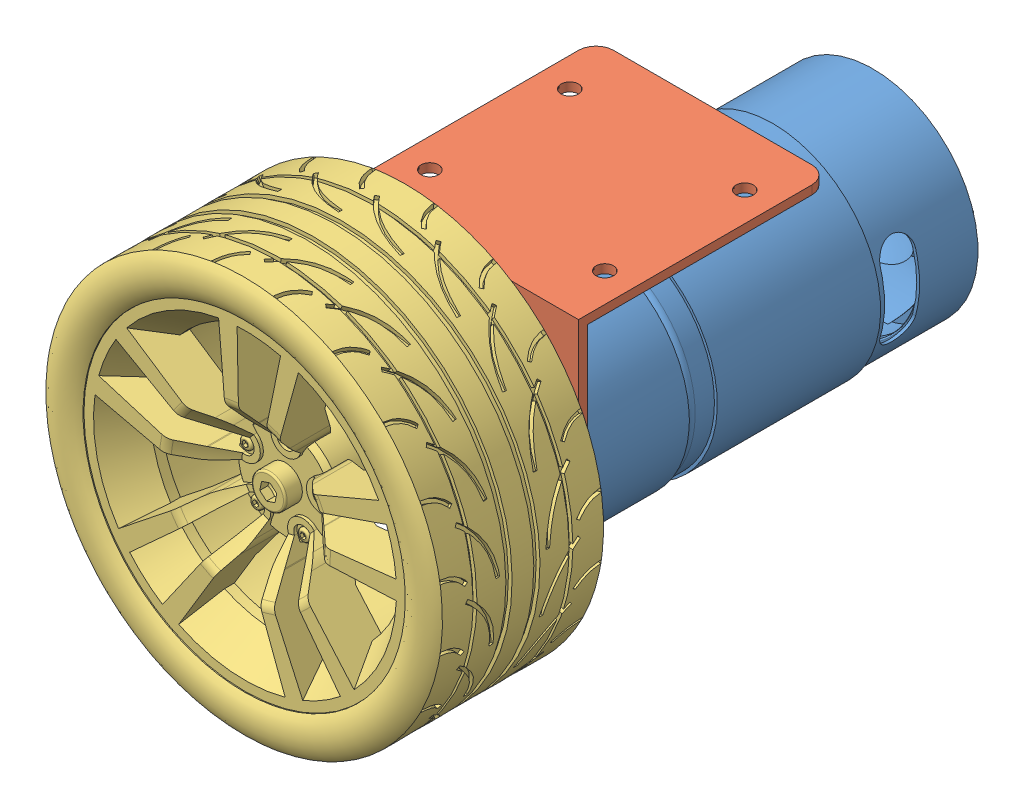
SolidWorks assembly assemblage_motor_complet, configuration Default. Lengths in mm.
Overall size (92.56 92.56 113.78).
4 component instances, 4 part files, 8 mates.
Components (placement in the parent):
- Motor 300RPM-1: Motor 300RPM [Default] at (60.9586 47.2064 18.9845) size (37 37 94.88)
- BAse-motor-1: BAse-motor [Predeterminado] at (28.5836 74.7064 94.3595) x (1 0 0) z (0 0 -1) size (40 46 43)
- wheel-1: wheel [Default] at (48.5836 55.7064 86.8847) x (-0.872522 -0.488575 0) z (-0.488575 0.872522 0) size (68 29.75 68)
- accoupelement court-1: accoupelement court [Default] at (48.5836 55.7064 101.8595) x (-0.320714 0.947176 0) z (0 0 1) size (13.86 12 18)
Mates (geometry in assembly coordinates):
- Coincident1: coincident anti-aligned: plane of Motor 300RPM-1 through (48.5836 48.7064 92.8595) normal (0 0 1); plane of BAse motor-1 through (48.5836 48.7064 92.8595) normal (0 0 -1)
- Concentric12: concentric anti-aligned: cylinder of Motor 300RPM-1 through (48.5836 48.7064 92.8595) axis (0 0 -1) radius 18.5; cylinder of BAse motor-1 through (48.5836 48.7064 92.8595) axis (0 0 1) radius 20
- Concentric13: concentric aligned: cylinder of Motor 300RPM-1 through (48.5836 55.7064 98.8595) axis (0 0 -1) radius 6; cylinder of BAse motor-1 through (48.5836 55.7064 134.3595) axis (0 0 -1) radius 6.4
- Concentric14: concentric aligned: cylinder of Motor 300RPM-1 through (48.5836 55.7064 113.8595) axis (0 0 -1) radius 3; cylinder of accoupelement court-1 through (48.5836 55.7064 113.8595) axis (0 0 -1) radius 3
- Coincident2: coincident anti-aligned: plane of Motor 300RPM-1 through (48.5836 55.7064 113.8595) normal (0 0 1); plane of accoupelement court-1 through (48.5836 55.7064 113.8595) normal (0 0 -1)
- Concentric15: concentric aligned: cylinder of wheel-1 through (48.5836 55.7064 131.6972) axis (0 0 -1) radius 34; cylinder of accoupelement court-1 through (48.5836 55.7064 113.8595) axis (0 0 -1) radius 5.75
- Coincident3: coincident anti-aligned: plane of wheel-1 through (48.5836 55.7064 119.8595) normal (0 0 -1); plane of accoupelement court-1 through (48.5836 55.7064 119.8595) normal (0 0 1)
- Parallel6: parallel anti-aligned: plane of wheel-1 through (56.4038 54.1446 119.8595) normal (-0.751335 0.659921 0); plane of accoupelement court-1 through (50.8056 49.1442 119.8595) normal (0.751335 -0.659921 0)
